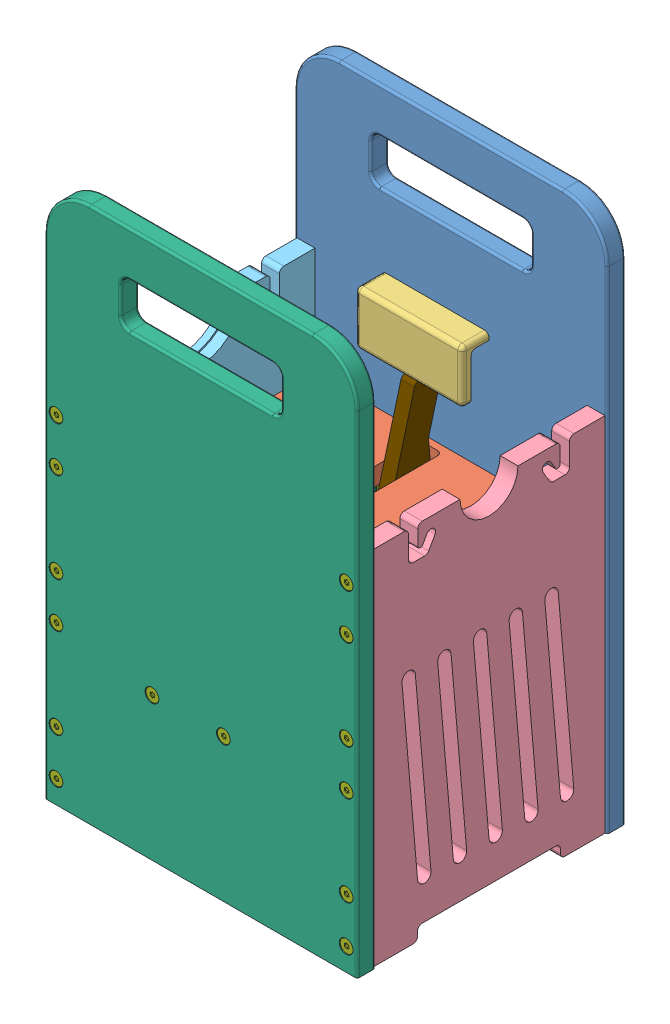
SolidWorks assembly R_ASSY_000_rev3, configuration Default. Lengths in mm.
Overall size (222.25 381 190.5).
147 component instances, 41 part files, 16 mates.
Components (placement in the parent):
- R_ASSY_100_Rev3-1: R_ASSY_100_Rev3 [Default] at origin size (222.25 381 190.5)
  - R_100_04_rev3-2: R_100_04_rev3 [Default] at origin size (222.25 381 12.7)
  - R_100_01_rev3-1: R_100_01_rev3 [Default] at (0 -16.002 95.25) x (-1 0 0) z (0 0 -1) size (193.68 12.7 175.26)
  - R_100_02_rev3-1: R_100_02_rev3 [Default] at (0 -171.577 95.25) x (-1 0 0) z (0 0 -1) size (198.44 12.7 175.26)
  - R_100_05 rev3-1: R_100_05 rev3 [Default] at (103.1875 -61.9125 95.25) x (0 0 1) z (-1 0 0) size (165.1 257.18 12.7)
  - R_100_06 rev3-1: R_100_06 rev3 [Default] at (-103.1875 -61.9125 95.25) x (0 0 1) z (-1 0 0) size (165.1 257.18 12.7)
  - R_100_03_rev3-2: R_100_03_rev3 [Default] at (0 0 190.5) x (-1 0 0) z (0 0 -1) size (222.25 381 12.7)
  - 95893A950_THREAD-FORMING TORX SCREW FOR PLASTICS-1: 95893A950_THREAD-FORMING TORX SCREW FOR PLASTICS [95893A950] at (-103.1875 49.5 172.8158) size (9.19 9.19 32.54)
  - 95893A950_THREAD-FORMING TORX SCREW FOR PLASTICS-2: 95893A950_THREAD-FORMING TORX SCREW FOR PLASTICS [95893A950] at (-103.1875 49.5 17.6842) x (-0.173648 0.984808 0) z (0 0 -1) size (9.19 9.19 32.54)
  - 95893A950_THREAD-FORMING TORX SCREW FOR PLASTICS-4: 95893A950_THREAD-FORMING TORX SCREW FOR PLASTICS [95893A950] at (103.1875 -174.5 17.6842) x (-0.173648 0.984808 0) z (0 0 -1) size (9.19 9.19 32.54)
  - 95893A950_THREAD-FORMING TORX SCREW FOR PLASTICS-5: 95893A950_THREAD-FORMING TORX SCREW FOR PLASTICS [95893A950] at (103.1875 49.5 17.6842) x (-0.173648 0.984808 0) z (0 0 -1) size (9.19 9.19 32.54)
  - 95893A950_THREAD-FORMING TORX SCREW FOR PLASTICS-6: 95893A950_THREAD-FORMING TORX SCREW FOR PLASTICS [95893A950] at (-103.1875 17.5 17.6842) x (-0.173648 0.984808 0) z (0 0 -1) size (9.19 9.19 32.54)
  - 95893A950_THREAD-FORMING TORX SCREW FOR PLASTICS-7: 95893A950_THREAD-FORMING TORX SCREW FOR PLASTICS [95893A950] at (103.1875 17.5 17.6842) x (-0.173648 0.984808 0) z (0 0 -1) size (9.19 9.19 32.54)
  - 95893A950_THREAD-FORMING TORX SCREW FOR PLASTICS-8: 95893A950_THREAD-FORMING TORX SCREW FOR PLASTICS [95893A950] at (-103.1875 -46.5 17.6842) x (-0.173648 0.984808 0) z (0 0 -1) size (9.19 9.19 32.54)
  - 95893A950_THREAD-FORMING TORX SCREW FOR PLASTICS-9: 95893A950_THREAD-FORMING TORX SCREW FOR PLASTICS [95893A950] at (103.1875 -46.5 17.6842) x (-0.173648 0.984808 0) z (0 0 -1) size (9.19 9.19 32.54)
  - 95893A950_THREAD-FORMING TORX SCREW FOR PLASTICS-10: 95893A950_THREAD-FORMING TORX SCREW FOR PLASTICS [95893A950] at (-103.1875 -78.5 17.6842) x (-0.173648 0.984808 0) z (0 0 -1) size (9.19 9.19 32.54)
  - 95893A950_THREAD-FORMING TORX SCREW FOR PLASTICS-11: 95893A950_THREAD-FORMING TORX SCREW FOR PLASTICS [95893A950] at (103.1875 -78.5 17.6842) x (-0.173648 0.984808 0) z (0 0 -1) size (9.19 9.19 32.54)
  - 95893A950_THREAD-FORMING TORX SCREW FOR PLASTICS-12: 95893A950_THREAD-FORMING TORX SCREW FOR PLASTICS [95893A950] at (-103.1875 -142.5 17.6842) x (-0.173648 0.984808 0) z (0 0 -1) size (9.19 9.19 32.54)
  - 95893A950_THREAD-FORMING TORX SCREW FOR PLASTICS-13: 95893A950_THREAD-FORMING TORX SCREW FOR PLASTICS [95893A950] at (103.1875 -142.5 17.6842) x (-0.173648 0.984808 0) z (0 0 -1) size (9.19 9.19 32.54)
  - 95893A950_THREAD-FORMING TORX SCREW FOR PLASTICS-14: 95893A950_THREAD-FORMING TORX SCREW FOR PLASTICS [95893A950] at (-34.925 -88.9 17.6842) x (-0.173648 0.984808 0) z (0 0 -1) size (9.19 9.19 32.54)
  - 95893A950_THREAD-FORMING TORX SCREW FOR PLASTICS-15: 95893A950_THREAD-FORMING TORX SCREW FOR PLASTICS [95893A950] at (15.875 -88.9 17.6842) x (-0.173648 0.984808 0) z (0 0 -1) size (9.19 9.19 32.54)
  - 95893A950_THREAD-FORMING TORX SCREW FOR PLASTICS-16: 95893A950_THREAD-FORMING TORX SCREW FOR PLASTICS [95893A950] at (-103.1875 -174.5 17.6842) x (-0.173648 0.984808 0) z (0 0 -1) size (9.19 9.19 32.54)
  - 95893A950_THREAD-FORMING TORX SCREW FOR PLASTICS-17: 95893A950_THREAD-FORMING TORX SCREW FOR PLASTICS [95893A950] at (103.1875 49.5 172.8158) size (9.19 9.19 32.54)
  - 95893A950_THREAD-FORMING TORX SCREW FOR PLASTICS-18: 95893A950_THREAD-FORMING TORX SCREW FOR PLASTICS [95893A950] at (-103.1875 -174.5 172.8158) size (9.19 9.19 32.54)
  - 95893A950_THREAD-FORMING TORX SCREW FOR PLASTICS-19: 95893A950_THREAD-FORMING TORX SCREW FOR PLASTICS [95893A950] at (103.1875 17.5 172.8158) size (9.19 9.19 32.54)
  - 95893A950_THREAD-FORMING TORX SCREW FOR PLASTICS-20: 95893A950_THREAD-FORMING TORX SCREW FOR PLASTICS [95893A950] at (-103.1875 17.5 172.8158) size (9.19 9.19 32.54)
  - 95893A950_THREAD-FORMING TORX SCREW FOR PLASTICS-21: 95893A950_THREAD-FORMING TORX SCREW FOR PLASTICS [95893A950] at (103.1875 -46.5 172.8158) size (9.19 9.19 32.54)
  - 95893A950_THREAD-FORMING TORX SCREW FOR PLASTICS-22: 95893A950_THREAD-FORMING TORX SCREW FOR PLASTICS [95893A950] at (-103.1875 -46.5 172.8158) size (9.19 9.19 32.54)
  - 95893A950_THREAD-FORMING TORX SCREW FOR PLASTICS-23: 95893A950_THREAD-FORMING TORX SCREW FOR PLASTICS [95893A950] at (103.1875 -78.5 172.8158) size (9.19 9.19 32.54)
  - 95893A950_THREAD-FORMING TORX SCREW FOR PLASTICS-24: 95893A950_THREAD-FORMING TORX SCREW FOR PLASTICS [95893A950] at (-103.1875 -78.5 172.8158) size (9.19 9.19 32.54)
  - 95893A950_THREAD-FORMING TORX SCREW FOR PLASTICS-25: 95893A950_THREAD-FORMING TORX SCREW FOR PLASTICS [95893A950] at (103.1875 -142.5 172.8158) size (9.19 9.19 32.54)
  - 95893A950_THREAD-FORMING TORX SCREW FOR PLASTICS-26: 95893A950_THREAD-FORMING TORX SCREW FOR PLASTICS [95893A950] at (-103.1875 -142.5 172.8158) size (9.19 9.19 32.54)
  - 95893A950_THREAD-FORMING TORX SCREW FOR PLASTICS-27: 95893A950_THREAD-FORMING TORX SCREW FOR PLASTICS [95893A950] at (15.875 -88.9 172.8158) size (9.19 9.19 32.54)
  - 95893A950_THREAD-FORMING TORX SCREW FOR PLASTICS-28: 95893A950_THREAD-FORMING TORX SCREW FOR PLASTICS [95893A950] at (-34.925 -88.9 172.8158) size (9.19 9.19 32.54)
  - 95893A950_THREAD-FORMING TORX SCREW FOR PLASTICS-29: 95893A950_THREAD-FORMING TORX SCREW FOR PLASTICS [95893A950] at (103.1875 -174.5 172.8158) size (9.19 9.19 32.54)
- R_ASSY_200_rev3-1: R_ASSY_200_rev3 [Default] at (132.6055 -209.5473 52.7848) x (0 0 1) z (-1 0 0) size (165.1 249.75 130.56)
  - R_200_01_rev3-1: R_200_01_rev3 [Default] at (42.4652 115.7578 110.3805) size (165.1 155.57 12.7)
  - STP-MTR-17048E-1: STP-MTR-17048E [Default] at (114.3442 119.6359 5.7474) x (-1 0 0) z (0 0 1) size (42.16 62.89 84.58)
  - R_200_03_rev2-1: R_200_03_rev2 [Default] at (39.2022 113.0052 142.1305) x (-0.709234 0.704973 0) z (0 0 1) size (6.35 6.35 50.8)
  - R_200_04-1: R_200_04 [Default] at (-14.6848 152.2703 142.1305) x (0.39149 -0.920182 0) z (0 0 -1) size (9.53 9.53 50.8)
  - R_200_04-2: R_200_04 [Default] at (99.6152 152.2703 142.1305) x (0.332871 0.942972 0) z (0 0 1) size (9.53 9.53 50.8)
  - 91116A120_TYPE 18-8 STAINLESS STL OVERSIZED FLAT WASHER-1: 91116A120_TYPE 18-8 STAINLESS STL OVERSIZED FLAT WASHER [91116A120] at (-20.6538 89.9768 116.7305) size (9 9 0.9)
  - 91116A120_TYPE 18-8 STAINLESS STL OVERSIZED FLAT WASHER-9: 91116A120_TYPE 18-8 STAINLESS STL OVERSIZED FLAT WASHER [91116A120] at (105.5842 89.9768 116.7305) x (0.949722 0.313094 0) z (0 0 1) size (9 9 0.9)
  - 91116A120_TYPE 18-8 STAINLESS STL OVERSIZED FLAT WASHER-11: 91116A120_TYPE 18-8 STAINLESS STL OVERSIZED FLAT WASHER [91116A120] at (105.5842 58.9888 116.7305) x (0.902124 0.431476 0) z (0 0 1) size (9 9 0.9)
  - 12t_Steel_Spur_Gear_32_DP_RS775_Motor_217-5859.step-1: 12t_Steel_Spur_Gear_32_DP_RS775_Motor_217-5859.step [Default] at (4.3652 69.7203 125.1283) size (10.98 10.98 19.05)
  - 12t_Steel_Spur_Gear_32_DP_RS775_Motor_217-5859.step-2: 12t_Steel_Spur_Gear_32_DP_RS775_Motor_217-5859.step [Default] at (74.0391 69.7203 125.1283) size (10.98 10.98 19.05)
  - R_200_05-1: R_200_05 [Default] at (39.2022 113.0052 132.6055) x (-0.958932 0.283637 0) z (0 0 -1) size (103.19 103.19 25.4)
  - R_200_02_rev3-1: R_200_02_rev3 [Default] at (42.4652 115.7578 161.1805) size (165.1 155.57 12.7)
  - R_200_07_SPCR_rev3-1: R_200_07_SPCR_rev3 [Default] at (39.2022 113.0052 153.243) size (12.7 12.7 7.68)
  - R_200_09_SPCR_rev3-3: R_200_09_SPCR_rev3 [Default] at (-14.6848 152.2703 135.7805) x (1 0 0) z (0 0 -1) size (17.46 17.46 12.57)
  - R_203_01_rev4-1: R_203_01_rev4 [Default] at (-14.6848 152.2703 142.1305) size (82.51 177.51 9.53)
  - R_200_09_SPCR_rev3-4: R_200_09_SPCR_rev3 [Default] at (99.6152 152.2703 123.2075) x (0.999677 -0.025413 0) z (0 0 1) size (17.46 17.46 12.57)
  - R_203_02_rev4-1: R_203_02_rev4 [Default] at (99.6152 152.2703 142.1305) x (-1 0 0) z (0 0 -1) size (82.48 176.02 9.53)
  - STP-MTR-17048E-2: STP-MTR-17048E [Default] at (44.6703 119.6359 5.7474) x (-1 0 0) z (0 0 1) size (42.16 62.89 84.58)
  - 91125A453_18-8 SS FEM THRDED ROUND STANDOFF-1: 91125A453_18-8 SS FEM THRDED ROUND STANDOFF [91125A453] at (-32.103 275.0161 142.1305) x (-1 0 0) z (0 0 1) size (6.35 6.35 10.62)
  - 91125A453_18-8 SS FEM THRDED ROUND STANDOFF-2: 91125A453_18-8 SS FEM THRDED ROUND STANDOFF [91125A453] at (-32.103 255.9661 142.1305) x (-0.987351 -0.158553 0) z (0 0 1) size (6.35 6.35 10.62)
  - 91125A453_18-8 SS FEM THRDED ROUND STANDOFF-4: 91125A453_18-8 SS FEM THRDED ROUND STANDOFF [91125A453] at (117.0334 275.0161 142.1305) x (-0.34202 0.939693 0) z (0 0 -1) size (6.35 6.35 10.62)
  - 91125A453_18-8 SS FEM THRDED ROUND STANDOFF-6: 91125A453_18-8 SS FEM THRDED ROUND STANDOFF [91125A453] at (117.0334 255.9661 142.1305) x (-0.5 0.866025 0) z (0 0 -1) size (6.35 6.35 10.62)
  - R_203_05-1: R_203_05 [Default] at (-28.928 268.6661 142.1305) x (0 0 -1) z (1 0 0) size (76.2 38.1 19.05)
  - 92949A192_18-8 SS BUTTON HEAD HEX DRIVE SCREW-19: 92949A192_18-8 SS BUTTON HEAD HEX DRIVE SCREW [92949A192] at (-32.103 275.0161 147.9979) x (-0.998312 -0.058087 0) z (0 0 1) size (7.92 7.92 12.15)
  - 92949A192_18-8 SS BUTTON HEAD HEX DRIVE SCREW-20: 92949A192_18-8 SS BUTTON HEAD HEX DRIVE SCREW [92949A192] at (-32.103 255.9661 147.9979) x (-0.976474 -0.215637 0) z (0 0 1) size (7.92 7.92 12.15)
  - 92949A192_18-8 SS BUTTON HEAD HEX DRIVE SCREW-22: 92949A192_18-8 SS BUTTON HEAD HEX DRIVE SCREW [92949A192] at (-32.103 275.0161 136.2631) x (0.973943 -0.226793 0) z (0 0 -1) size (7.92 7.92 12.15)
  - 92949A192_18-8 SS BUTTON HEAD HEX DRIVE SCREW-25: 92949A192_18-8 SS BUTTON HEAD HEX DRIVE SCREW [92949A192] at (-32.103 255.9661 136.2631) x (0.948563 -0.316589 0) z (0 0 -1) size (7.92 7.92 12.15)
  - 92949A192_18-8 SS BUTTON HEAD HEX DRIVE SCREW-27: 92949A192_18-8 SS BUTTON HEAD HEX DRIVE SCREW [92949A192] at (117.0334 275.0161 147.9979) x (-0.973943 -0.226793 0) z (0 0 1) size (7.92 7.92 12.15)
  - 92949A192_18-8 SS BUTTON HEAD HEX DRIVE SCREW-28: 92949A192_18-8 SS BUTTON HEAD HEX DRIVE SCREW [92949A192] at (117.0334 255.9661 147.9979) x (-0.948563 -0.316589 0) z (0 0 1) size (7.92 7.92 12.15)
  - 92949A192_18-8 SS BUTTON HEAD HEX DRIVE SCREW-29: 92949A192_18-8 SS BUTTON HEAD HEX DRIVE SCREW [92949A192] at (117.0334 275.0161 136.2631) x (-0.998312 0.058087 0) z (0 0 -1) size (7.92 7.92 12.15)
  - 92949A192_18-8 SS BUTTON HEAD HEX DRIVE SCREW-30: 92949A192_18-8 SS BUTTON HEAD HEX DRIVE SCREW [92949A192] at (117.0334 255.9661 136.2631) x (-0.976474 0.215637 0) z (0 0 -1) size (7.92 7.92 12.15)
  - R_203_05-2: R_203_05 [Default] at (113.8584 268.6661 142.1305) x (0 0 1) z (-1 0 0) size (76.2 38.1 19.05)
  - 2797T100_LIGHT DUTY DRY-RUNNING THRUST BEARING-1: 2797T100_LIGHT DUTY DRY-RUNNING THRUST BEARING [2797T1] at (39.2022 113.0052 123.8742) x (-0.703019 0.711171 0) z (0 0 1) size (15.88 15.88 1.59)
  - 6338K413_OIL-EMBEDDED FLANGED SLEEVE BEARING-1: 6338K413_OIL-EMBEDDED FLANGED SLEEVE BEARING [6338K413] at (39.2022 113.0052 124.668) x (1 0 0) z (0 -1 0) size (12.7 12.7 12.7)
  - 6338K413_OIL-EMBEDDED FLANGED SLEEVE BEARING-2: 6338K413_OIL-EMBEDDED FLANGED SLEEVE BEARING [6338K413] at (39.2022 113.0052 153.243) x (0.987351 -0.158553 0) z (0.158553 0.987351 0) size (12.7 12.7 12.7)
  - 6338K414_OIL-EMBEDDED FLANGED SLEEVE BEARING-1: 6338K414_OIL-EMBEDDED FLANGED SLEEVE BEARING [6338K414] at (-14.6848 152.2703 135.7805) x (0.998098 0.061654 0) z (0.061654 -0.998098 0) size (17.46 6.35 17.46)
  - 6338K414_OIL-EMBEDDED FLANGED SLEEVE BEARING-2: 6338K414_OIL-EMBEDDED FLANGED SLEEVE BEARING [6338K414] at (-14.6848 152.2703 148.4805) x (0.995248 -0.097377 0) z (0.097377 0.995248 0) size (17.46 6.35 17.46)
  - 6338K414_OIL-EMBEDDED FLANGED SLEEVE BEARING-4: 6338K414_OIL-EMBEDDED FLANGED SLEEVE BEARING [6338K414] at (99.6152 152.2703 148.4805) x (-0.283434 0.958992 0) z (-0.958992 -0.283434 0) size (17.46 6.35 17.46)
  - 6338K414_OIL-EMBEDDED FLANGED SLEEVE BEARING-6: 6338K414_OIL-EMBEDDED FLANGED SLEEVE BEARING [6338K414] at (99.6152 152.2703 135.7805) x (-0.552443 -0.833551 0) z (-0.833551 0.552443 0) size (17.46 6.35 17.46)
  - R_200_09_SPCR_rev3-5: R_200_09_SPCR_rev3 [Default] at (99.6152 152.2703 161.0535) x (0.966573 0.25639 0) z (0 0 -1) size (17.46 17.46 12.57)
  - R_200_09_SPCR_rev3-7: R_200_09_SPCR_rev3 [Default] at (-14.6848 152.2703 161.0535) x (-0.36579 0.930697 0) z (0 0 -1) size (17.46 17.46 12.57)
  - 91116A120_TYPE 18-8 STAINLESS STL OVERSIZED FLAT WASHER-12: 91116A120_TYPE 18-8 STAINLESS STL OVERSIZED FLAT WASHER [91116A120] at (89.5331 85.2143 116.7305) size (9 9 0.9)
  - 91292A027_TYPE 18-8 SS SOCKET HEAD CAP SCREW-1: 91292A027_TYPE 18-8 SS SOCKET HEAD CAP SCREW [91292A027] at (89.5331 85.2143 103.6305) x (-0.923728 -0.383049 0) z (0 0 -1) size (5.5 5.5 17.24)
  - 91292A027_TYPE 18-8 SS SOCKET HEAD CAP SCREW-8: 91292A027_TYPE 18-8 SS SOCKET HEAD CAP SCREW [91292A027] at (89.5331 54.2263 103.6305) x (-0.923728 -0.383049 0) z (0 0 -1) size (5.5 5.5 17.24)
  - 91292A027_TYPE 18-8 SS SOCKET HEAD CAP SCREW-9: 91292A027_TYPE 18-8 SS SOCKET HEAD CAP SCREW [91292A027] at (-11.1288 85.2143 103.6305) x (-0.923728 -0.383049 0) z (0 0 -1) size (5.5 5.5 17.24)
  - 91292A027_TYPE 18-8 SS SOCKET HEAD CAP SCREW-10: 91292A027_TYPE 18-8 SS SOCKET HEAD CAP SCREW [91292A027] at (58.5451 85.2143 103.6305) x (-0.923728 -0.383049 0) z (0 0 -1) size (5.5 5.5 17.24)
  - 91292A027_TYPE 18-8 SS SOCKET HEAD CAP SCREW-11: 91292A027_TYPE 18-8 SS SOCKET HEAD CAP SCREW [91292A027] at (58.5451 54.2263 103.6305) x (-0.923728 -0.383049 0) z (0 0 -1) size (5.5 5.5 17.24)
  - 91292A027_TYPE 18-8 SS SOCKET HEAD CAP SCREW-12: 91292A027_TYPE 18-8 SS SOCKET HEAD CAP SCREW [91292A027] at (-11.1288 54.2263 103.6305) x (-0.923728 -0.383049 0) z (0 0 -1) size (5.5 5.5 17.24)
  - 91292A027_TYPE 18-8 SS SOCKET HEAD CAP SCREW-13: 91292A027_TYPE 18-8 SS SOCKET HEAD CAP SCREW [91292A027] at (19.8592 54.2263 103.6305) x (-0.923728 -0.383049 0) z (0 0 -1) size (5.5 5.5 17.24)
  - 91292A027_TYPE 18-8 SS SOCKET HEAD CAP SCREW-14: 91292A027_TYPE 18-8 SS SOCKET HEAD CAP SCREW [91292A027] at (19.8592 85.2143 103.6305) x (-0.923728 -0.383049 0) z (0 0 -1) size (5.5 5.5 17.24)
  - 91116A120_TYPE 18-8 STAINLESS STL OVERSIZED FLAT WASHER-19: 91116A120_TYPE 18-8 STAINLESS STL OVERSIZED FLAT WASHER [91116A120] at (89.5331 54.2263 116.7305) size (9 9 0.9)
  - 91116A120_TYPE 18-8 STAINLESS STL OVERSIZED FLAT WASHER-20: 91116A120_TYPE 18-8 STAINLESS STL OVERSIZED FLAT WASHER [91116A120] at (-11.1288 85.2143 116.7305) size (9 9 0.9)
  - 91116A120_TYPE 18-8 STAINLESS STL OVERSIZED FLAT WASHER-21: 91116A120_TYPE 18-8 STAINLESS STL OVERSIZED FLAT WASHER [91116A120] at (58.5451 85.2143 116.7305) size (9 9 0.9)
  - 91116A120_TYPE 18-8 STAINLESS STL OVERSIZED FLAT WASHER-22: 91116A120_TYPE 18-8 STAINLESS STL OVERSIZED FLAT WASHER [91116A120] at (58.5451 54.2263 116.7305) size (9 9 0.9)
  - 91116A120_TYPE 18-8 STAINLESS STL OVERSIZED FLAT WASHER-23: 91116A120_TYPE 18-8 STAINLESS STL OVERSIZED FLAT WASHER [91116A120] at (-11.1288 54.2263 116.7305) size (9 9 0.9)
  - 91116A120_TYPE 18-8 STAINLESS STL OVERSIZED FLAT WASHER-24: 91116A120_TYPE 18-8 STAINLESS STL OVERSIZED FLAT WASHER [91116A120] at (19.8592 54.2263 116.7305) size (9 9 0.9)
  - 91116A120_TYPE 18-8 STAINLESS STL OVERSIZED FLAT WASHER-25: 91116A120_TYPE 18-8 STAINLESS STL OVERSIZED FLAT WASHER [91116A120] at (19.8592 85.2143 116.7305) size (9 9 0.9)
  - dc1c-a1aa-1: dc1c-a1aa [Default] at (-27.4348 169.2553 154.8305) x (0 1 0) z (-1 0 0) size (19.85 14.96 6.45)
    - dc1c-a1aa_01-1: dc1c-a1aa_01 [Default] at origin size (5.58 3.61 5.58)
    - dc1c-a1aa_02-1: dc1c-a1aa_02 [Default] at origin size (19.73 5.96 6.26)
    - dc1c-a1aa_03-1: dc1c-a1aa_03 [Default] at origin size (19.85 3.9 6.45)
    - dc1c-a1aa_04-1: dc1c-a1aa_04 [Default] at origin size (1.69 3.85 2.68)
    - dc1c-a1aa_05-1: dc1c-a1aa_05 [Default] at origin size (1.69 3.85 2.68)
    - dc1c-a1aa_06-1: dc1c-a1aa_06 [Default] at origin size (1.69 3.85 2.68)
  - 92095A104_BUTTON HEAD HEX DRIVE SCREW-1: 92095A104_BUTTON HEAD HEX DRIVE SCREW [92095A104] at (-31.5598 169.2553 154.8305) x (0 0 1) z (-1 0 0) size (3.8 3.8 11.02)
  - R_200_10-2: R_200_10 [Default] at (-20.241 174.0203 167.5305) x (0 0 1) z (-1 0 0) size (14.29 19.05 9.53)
  - 92095A104_BUTTON HEAD HEX DRIVE SCREW-2: 92095A104_BUTTON HEAD HEX DRIVE SCREW [92095A104] at (-31.5598 178.7853 154.8305) x (0 -0.984808 -0.173648) z (-1 0 0) size (3.8 3.8 11.02)
  - R_200_10-3: R_200_10 [Default] at (-8.9998 130.5536 167.5305) x (0 0 1) z (-0.87462 -0.48481 0) size (14.29 19.05 9.53)
  - dc1c-a1aa-2: dc1c-a1aa [Default] at (-17.6017 131.2336 154.8305) x (0.48481 -0.87462 0) z (0.87462 0.48481 0) size (19.85 14.96 6.45)
    - dc1c-a1aa_01-1: dc1c-a1aa_01 [Default] at origin size (5.58 3.61 5.58)
    - dc1c-a1aa_02-1: dc1c-a1aa_02 [Default] at origin size (19.73 5.96 6.26)
    - dc1c-a1aa_03-1: dc1c-a1aa_03 [Default] at origin size (19.85 3.9 6.45)
    - dc1c-a1aa_04-1: dc1c-a1aa_04 [Default] at origin size (1.69 3.85 2.68)
    - dc1c-a1aa_05-1: dc1c-a1aa_05 [Default] at origin size (1.69 3.85 2.68)
    - dc1c-a1aa_06-1: dc1c-a1aa_06 [Default] at origin size (1.69 3.85 2.68)
  - 92095A104_BUTTON HEAD HEX DRIVE SCREW-3: 92095A104_BUTTON HEAD HEX DRIVE SCREW [92095A104] at (-21.2095 129.2337 154.8305) x (-0.34402 0.620628 0.704607) z (-0.87462 -0.48481 0) size (3.8 3.8 11.02)
  - 92095A104_BUTTON HEAD HEX DRIVE SCREW-5: 92095A104_BUTTON HEAD HEX DRIVE SCREW [92095A104] at (-16.5893 120.8986 154.8305) x (-0.449843 0.811539 -0.372887) z (-0.87462 -0.48481 0) size (3.8 3.8 11.02)
  - 92141A009_TYPE 18-8 STAINLESS STEEL FLAT WASHER-5: 92141A009_TYPE 18-8 STAINLESS STEEL FLAT WASHER [92141A009] at (-20.241 180.3703 174.8965) x (-0.777574 -0.628792 0) z (0.628792 -0.777574 0) size (9.53 1.02 9.53)
  - 92949A194_18-8 SS BUTTON HEAD HEX DRIVE SCREW-12: 92949A194_18-8 SS BUTTON HEAD HEX DRIVE SCREW [92949A194] at (-20.241 180.3703 169.6514) x (0.994367 -0.105992 0) z (0 0 1) size (7.92 7.92 15.34)
  - 92141A009_TYPE 18-8 STAINLESS STEEL FLAT WASHER-6: 92141A009_TYPE 18-8 STAINLESS STEEL FLAT WASHER [92141A009] at (-20.241 167.6703 174.8965) x (-0.668041 -0.744124 0) z (0.744124 -0.668041 0) size (9.53 1.02 9.53)
  - 92949A194_18-8 SS BUTTON HEAD HEX DRIVE SCREW-17: 92949A194_18-8 SS BUTTON HEAD HEX DRIVE SCREW [92949A194] at (-20.241 167.6703 169.6514) x (0.964983 -0.262311 0) z (0 0 1) size (7.92 7.92 15.34)
  - 92141A009_TYPE 18-8 STAINLESS STEEL FLAT WASHER-7: 92141A009_TYPE 18-8 STAINLESS STEEL FLAT WASHER [92141A009] at (-14.6848 152.2703 174.8965) x (-0.567853 -0.82313 0) z (0.82313 -0.567853 0) size (9.53 1.02 9.53)
  - 92949A194_18-8 SS BUTTON HEAD HEX DRIVE SCREW-18: 92949A194_18-8 SS BUTTON HEAD HEX DRIVE SCREW [92949A194] at (-14.6848 152.2703 169.6514) x (0.923728 -0.383049 0) z (0 0 1) size (7.92 7.92 15.34)
  - 92141A009_TYPE 18-8 STAINLESS STEEL FLAT WASHER-8: 92141A009_TYPE 18-8 STAINLESS STEEL FLAT WASHER [92141A009] at (-12.0783 136.1074 174.8965) x (-0.488654 -0.872477 0) z (0.872477 -0.488654 0) size (9.53 1.02 9.53)
  - 92949A194_18-8 SS BUTTON HEAD HEX DRIVE SCREW-19: 92949A194_18-8 SS BUTTON HEAD HEX DRIVE SCREW [92949A194] at (-12.0783 136.1074 169.6514) x (0.884001 -0.467484 0) z (0 0 1) size (7.92 7.92 15.34)
  - 92141A009_TYPE 18-8 STAINLESS STEEL FLAT WASHER-9: 92141A009_TYPE 18-8 STAINLESS STEEL FLAT WASHER [92141A009] at (-5.9212 124.9998 174.8965) x (-0.440433 -0.897785 0) z (0.897785 -0.440433 0) size (9.53 1.02 9.53)
  - 92949A194_18-8 SS BUTTON HEAD HEX DRIVE SCREW-20: 92949A194_18-8 SS BUTTON HEAD HEX DRIVE SCREW [92949A194] at (-5.9212 124.9998 169.6514) x (0.857241 -0.514915 0) z (0 0 1) size (7.92 7.92 15.34)
  - 92141A009_TYPE 18-8 STAINLESS STEEL FLAT WASHER-10: 92141A009_TYPE 18-8 STAINLESS STEEL FLAT WASHER [92141A009] at (39.2022 113.0052 174.8965) x (-0.431679 -0.902027 0) z (0.902027 -0.431679 0) size (9.53 1.02 9.53)
  - 92949A194_18-8 SS BUTTON HEAD HEX DRIVE SCREW-16: 92949A194_18-8 SS BUTTON HEAD HEX DRIVE SCREW [92949A194] at (39.2022 113.0052 169.6514) x (0.852192 -0.523229 0) z (0 0 1) size (7.92 7.92 15.34)
  - 92141A009_TYPE 18-8 STAINLESS STEEL FLAT WASHER-11: 92141A009_TYPE 18-8 STAINLESS STEEL FLAT WASHER [92141A009] at (99.6152 152.2703 174.8965) x (-0.468067 -0.883693 0) z (0.883693 -0.468067 0) size (9.53 1.02 9.53)
  - 92949A194_18-8 SS BUTTON HEAD HEX DRIVE SCREW-11: 92949A194_18-8 SS BUTTON HEAD HEX DRIVE SCREW [92949A194] at (99.6152 152.2703 169.6514) x (0.872799 -0.488079 0) z (0 0 1) size (7.92 7.92 15.34)
  - 92141A009_TYPE 18-8 STAINLESS STEEL FLAT WASHER-14: 92141A009_TYPE 18-8 STAINLESS STEEL FLAT WASHER [92141A009] at (-14.6848 152.2703 109.3645) x (-0.484215 -0.874949 0) z (-0.874949 0.484215 0) size (9.53 1.02 9.53)
  - 92949A194_18-8 SS BUTTON HEAD HEX DRIVE SCREW-22: 92949A194_18-8 SS BUTTON HEAD HEX DRIVE SCREW [92949A194] at (-14.6848 152.2703 114.6096) x (-0.277052 0.960855 0) z (0 0 -1) size (7.92 7.92 15.34)
  - 92141A009_TYPE 18-8 STAINLESS STEEL FLAT WASHER-16: 92141A009_TYPE 18-8 STAINLESS STEEL FLAT WASHER [92141A009] at (39.2022 113.0052 109.3645) x (-0.324925 -0.94574 0) z (-0.94574 0.324925 0) size (9.53 1.02 9.53)
  - 92949A194_18-8 SS BUTTON HEAD HEX DRIVE SCREW-24: 92949A194_18-8 SS BUTTON HEAD HEX DRIVE SCREW [92949A194] at (39.2022 113.0052 114.6096) x (-0.439693 0.898148 0) z (0 0 -1) size (7.92 7.92 15.34)
  - 92141A009_TYPE 18-8 STAINLESS STEEL FLAT WASHER-18: 92141A009_TYPE 18-8 STAINLESS STEEL FLAT WASHER [92141A009] at (99.6152 152.2703 109.3645) x (-0.155763 -0.987795 0) z (-0.987795 0.155763 0) size (9.53 1.02 9.53)
  - 92949A194_18-8 SS BUTTON HEAD HEX DRIVE SCREW-26: 92949A194_18-8 SS BUTTON HEAD HEX DRIVE SCREW [92949A194] at (99.6152 152.2703 114.6096) x (-0.588975 0.808151 0) z (0 0 -1) size (7.92 7.92 15.34)
  - 93365A142_HEAT-SET INSERTS FOR PLASTICS-1: 93365A142_HEAT-SET INSERTS FOR PLASTICS [93365A142] at (115.4902 114.0178 110.3805) x (-0.923728 -0.383049 0) z (0.383049 -0.923728 0) size (6.35 8.46 6.35)
  - 93365A142_HEAT-SET INSERTS FOR PLASTICS-2: 93365A142_HEAT-SET INSERTS FOR PLASTICS [93365A142] at (-30.5598 114.0178 110.3805) x (-0.923728 -0.383049 0) z (0.383049 -0.923728 0) size (6.35 8.46 6.35)
  - 93365A142_HEAT-SET INSERTS FOR PLASTICS-3: 93365A142_HEAT-SET INSERTS FOR PLASTICS [93365A142] at (-30.5598 164.0178 110.3805) x (-0.923728 -0.383049 0) z (0.383049 -0.923728 0) size (6.35 8.46 6.35)
  - 93365A142_HEAT-SET INSERTS FOR PLASTICS-4: 93365A142_HEAT-SET INSERTS FOR PLASTICS [93365A142] at (115.4902 164.0178 110.3805) x (-0.923728 -0.383049 0) z (0.383049 -0.923728 0) size (6.35 8.46 6.35)
- R_ASSY_300-1: R_ASSY_300 [Default] at (26.9875 -45.5295 95.25) x (0 0 -1) z (1 0 0) size (158.75 86 52.53)
  - R_300_01-1: R_300_01 [Default] x (0 1 0) z (-1 0 0) size (19.05 9.53 158.75)
  - RPS-400-48-C-1: RPS-400-48-C [Default] at (0 -25.3 26.2625) x (1 0 0) z (0 -1 0) size (130 43 86)
  - R_300_01-2: R_300_01 [Default] at (0 -50 0) x (0 1 0) z (-1 0 0) size (19.05 9.53 158.75)
  - 91116A120_TYPE 18-8 STAINLESS STL OVERSIZED FLAT WASHER-1: 91116A120_TYPE 18-8 STAINLESS STL OVERSIZED FLAT WASHER [91116A120] at (60 0 -1.6937) size (9 9 0.9)
  - 92095A181_BUTTON HEAD HEX DRIVE SCREW-1: 92095A181_BUTTON HEAD HEX DRIVE SCREW [92095A181] at (60 0 -3.3438) x (-0.923728 -0.383049 0) z (0 0 -1) size (5.7 5.7 9.83)
- 92949A196_18-8 SS BUTTON HEAD HEX DRIVE SCREW-1: 92949A196_18-8 SS BUTTON HEAD HEX DRIVE SCREW [92949A196] at (24.9174 -45.5295 168.275) x (0 0 -1) z (1 0 0) size (7.92 7.92 18.54)
- 92949A196_18-8 SS BUTTON HEAD HEX DRIVE SCREW-2: 92949A196_18-8 SS BUTTON HEAD HEX DRIVE SCREW [92949A196] at (24.9174 -45.5295 22.225) x (0 0 -1) z (1 0 0) size (7.92 7.92 18.54)
- 92949A196_18-8 SS BUTTON HEAD HEX DRIVE SCREW-3: 92949A196_18-8 SS BUTTON HEAD HEX DRIVE SCREW [92949A196] at (24.9174 -95.5295 22.225) x (0 0 -1) z (1 0 0) size (7.92 7.92 18.54)
- 92949A196_18-8 SS BUTTON HEAD HEX DRIVE SCREW-4: 92949A196_18-8 SS BUTTON HEAD HEX DRIVE SCREW [92949A196] at (24.9174 -95.5295 168.275) x (0 0 -1) z (1 0 0) size (7.92 7.92 18.54)
Mates (geometry in assembly coordinates):
- Width1: width: plane of R_ASSY_200_rev3-1/R_200_01_rev3-1 through (9.525 -22.352 12.7) normal (0 1 0); plane of R_ASSY_200_rev3-1/R_200_01_rev3-1 through (9.525 -165.227 12.7) normal (0 -1 0); plane of R_ASSY_100_Rev3-1/R_100_02_rev3-1 through (-96.8375 -165.227 7.62) normal (0 1 0); plane of R_ASSY_100_Rev3-1/R_100_01_rev3-1 through (-96.8375 -22.352 7.62) normal (0 -1 0)
- Width2: width: plane of R_ASSY_100_Rev3-1/R_100_02_rev3-1 through (22.352 -177.927 143.002) normal (-1 0 0); plane of R_ASSY_100_Rev3-1/R_100_02_rev3-1 through (-41.402 -177.927 130.302) normal (1 0 0); plane of R_ASSY_200_rev3-1/R_200_01_rev3-1 through (22.225 -93.7895 95.25) normal (1 0 0); plane of R_ASSY_200_rev3-1/R_200_02_rev3-1 through (-41.275 -93.7895 95.25) normal (-1 0 0)
- Width3: width: plane of R_ASSY_100_Rev3-1/R_100_02_rev3-1 through (22.352 -177.927 158.877) normal (0 0 -1); plane of R_ASSY_100_Rev3-1/R_100_02_rev3-1 through (22.352 -177.927 31.623) normal (0 0 1); plane of R_ASSY_200_rev3-1/R_200_01_rev3-1 through (45.3393 -165.227 158.75) normal (0 0 1); plane of R_ASSY_200_rev3-1/R_200_01_rev3-1 through (45.3393 -165.227 31.75) normal (0 0 -1)
- Coincident1: coincident: plane of R_ASSY_200_rev3-1/R_200_01_rev3-1 through (22.225 -93.7895 95.25) normal (1 0 0); plane of R_ASSY_300-1/R_300_01-1 through (22.225 -55.0545 174.625) normal (-1 0 0)
- Concentric1: concentric: cylinder of R_ASSY_200_rev3-1/R_200_01_rev3-1 through (22.225 -45.5295 168.275) axis (1 0 0) radius 2.6098; cylinder of R_ASSY_300-1/R_300_01-1 through (22.225 -45.5295 168.275) axis (-1 0 0) radius 2.2479
- Concentric2: concentric: cylinder of R_ASSY_200_rev3-1/R_200_01_rev3-1 through (22.225 -45.5295 22.225) axis (1 0 0) radius 2.6098; cylinder of R_ASSY_300-1/R_300_01-1 through (22.225 -45.5295 22.225) axis (-1 0 0) radius 2.2479
- Concentric3: concentric: cylinder of R_ASSY_200_rev3-1/R_200_01_rev3-1 through (22.225 -95.5295 22.225) axis (1 0 0) radius 2.6098; cylinder of R_ASSY_300-1/R_300_01-2 through (22.225 -95.5295 22.225) axis (-1 0 0) radius 2.2479
- Concentric4: concentric: cylinder of R_ASSY_200_rev3-1/R_200_01_rev3-1 through (22.225 -95.5295 168.275) axis (1 0 0) radius 2.6098; cylinder of R_ASSY_300-1/R_300_01-2 through (22.225 -95.5295 168.275) axis (-1 0 0) radius 2.2479
- Coincident3: coincident: plane of R_ASSY_300-1/R_300_01-1 through (31.75 -55.0545 174.625) normal (1 0 0); plane of 92949A196_18-8 SS BUTTON HEAD HEX DRIVE SCREW-1 through (31.75 -41.5671 168.275) normal (-1 0 0)
- Concentric6: concentric: cylinder of R_ASSY_300-1/R_300_01-1 through (22.225 -45.5295 168.275) axis (-1 0 0) radius 2.2479; cylinder of 92949A196_18-8 SS BUTTON HEAD HEX DRIVE SCREW-1 through (33.9598 -45.5295 168.275) axis (1 0 0) radius 3.9624
- Coincident4: coincident: plane of R_ASSY_300-1/R_300_01-2 through (31.75 -105.0545 174.625) normal (1 0 0); plane of 92949A196_18-8 SS BUTTON HEAD HEX DRIVE SCREW-4 through (31.75 -91.5671 168.275) normal (-1 0 0)
- Concentric7: concentric: cylinder of R_ASSY_300-1/R_300_01-2 through (22.225 -95.5295 168.275) axis (-1 0 0) radius 2.2479; cylinder of 92949A196_18-8 SS BUTTON HEAD HEX DRIVE SCREW-4 through (33.9598 -95.5295 168.275) axis (1 0 0) radius 3.9624
- Coincident5: coincident: plane of R_ASSY_300-1/R_300_01-2 through (31.75 -105.0545 174.625) normal (1 0 0); plane of 92949A196_18-8 SS BUTTON HEAD HEX DRIVE SCREW-3 through (31.75 -91.5671 22.225) normal (-1 0 0)
- Concentric8: concentric: cylinder of R_ASSY_300-1/R_300_01-2 through (22.225 -95.5295 22.225) axis (-1 0 0) radius 2.2479; cylinder of 92949A196_18-8 SS BUTTON HEAD HEX DRIVE SCREW-3 through (33.9598 -95.5295 22.225) axis (1 0 0) radius 3.9624
- Coincident6: coincident: plane of R_ASSY_300-1/R_300_01-1 through (31.75 -55.0545 174.625) normal (1 0 0); plane of 92949A196_18-8 SS BUTTON HEAD HEX DRIVE SCREW-2 through (31.75 -41.5671 22.225) normal (-1 0 0)
- Concentric9: concentric: cylinder of R_ASSY_300-1/R_300_01-1 through (22.225 -45.5295 22.225) axis (-1 0 0) radius 2.2479; cylinder of 92949A196_18-8 SS BUTTON HEAD HEX DRIVE SCREW-2 through (33.9598 -45.5295 22.225) axis (1 0 0) radius 3.9624
